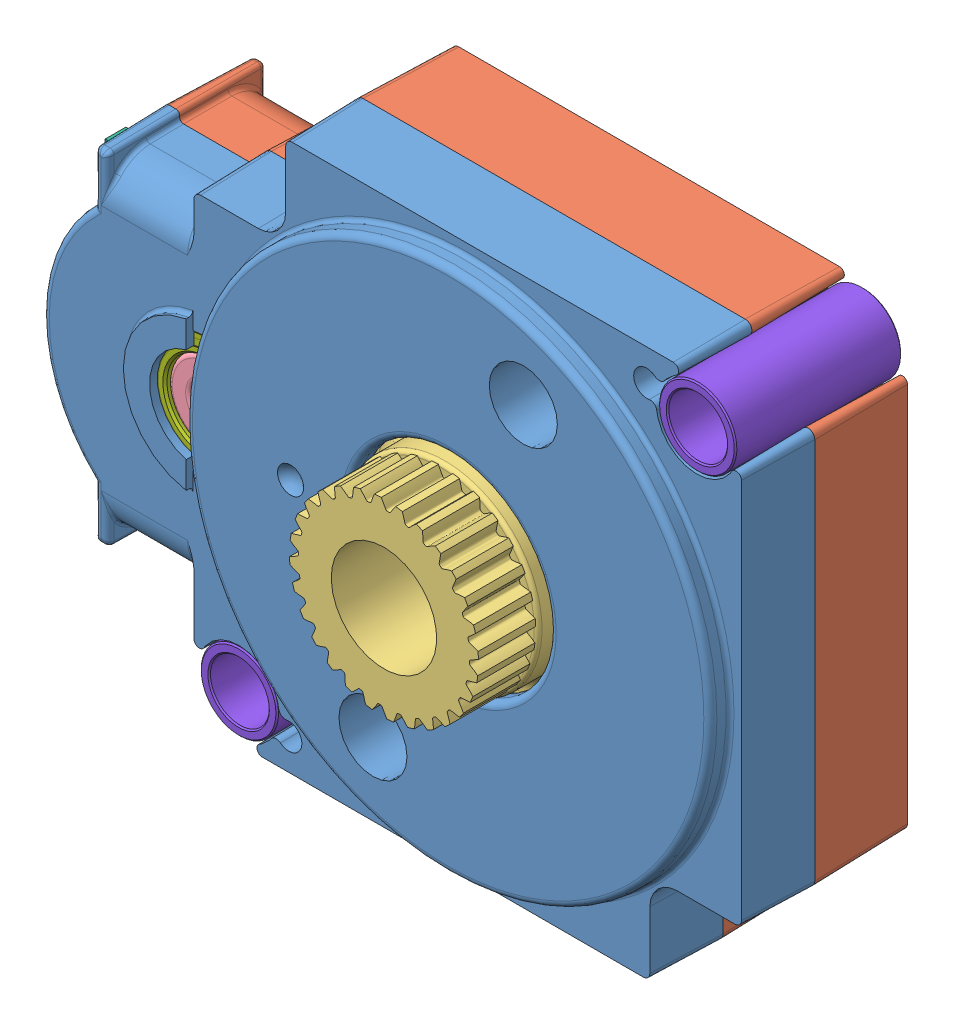
SolidWorks assembly 217-5046-STEP-201512011, configuration Default. Lengths in mm.
Overall size (58.21 43.13 22.65).
11 component instances, 10 part files, 0 mates.
Components (placement in the parent):
- 217-4783-001 Rev3-1: 217-4783-001 Rev3 [Default] at (0 0 2.75) size (53.55 42 11.11)
- 217-4783-002 Rev7_Sealed Config_1-1: 217-4783-002 Rev7_Sealed Config_1 [Default] at (0 0 -7.2) x (0 1 0) z (0 0 1) size (42 51.56 9.32)
- 217-4783-005 Rev7_40t_spur_REF_14deg_1-1: 217-4783-005 Rev7_40t_spur_REF_14deg_1 [Default] at (0 0 5.95) x (0.660339 0.750968 0) z (0 0 1) size (21.16 21.1 17.1)
- 217-4783-004 Rev2_40t_spur_REF_14deg_1-1: 217-4783-004 Rev2_40t_spur_REF_14deg_1 [Default] at (-20.05 0 5.2) x (-0.718289 0.695745 0) z (0 0 1) size (21.07 21.07 4.88)
- 217-4783-008 Rev2_1-1: 217-4783-008 Rev2_1 [Default] at (-20.05 0 2.2) x (0.307149 -0.951661 0) z (0.951661 0.307149 0) size (5 4 5)
- PCBA Rev3-1: PCBA Rev3 [Default] at (-20.05 0 -2.1252) x (0 1 0) z (-1 0 0) size (15.93 10.15 24.58)
- 217-2788-001 Rev3_57155K375_1-1: 217-2788-001 Rev3_57155K375_1 [Default] at (-20.05 0 3.8125) x (-0.99574 0.092202 0) z (0 0 1) size (9.53 9.53 3.17)
- 217-4783-006 Rev3_1-1: 217-4783-006 Rev3_1 [Default] at (17.5 17.5 -0.85) x (-0.867641 0.497191 0) z (0 0 1) size (5.9 5.9 12.7)
- 217-4783-006 Rev3_1-2: 217-4783-006 Rev3_1 [Default] at (-17.5 -17.5 -0.85) x (0.825154 -0.564908 0) z (0 0 1) size (5.9 5.9 12.7)
- 217-4783-007 Rev1_1-1: 217-4783-007 Rev1_1 [Default] at (-16.45 0 -5.2) x (0 1 0) z (0 0 1) size (6 10.71 3.56)
- 217-4783-003 Rev4_1-1: 217-4783-003 Rev4_1 [Default] at (-20.05 0 -1.02) x (0 1 0) z (0 0 1) size (23.4 21.71 4.21)
